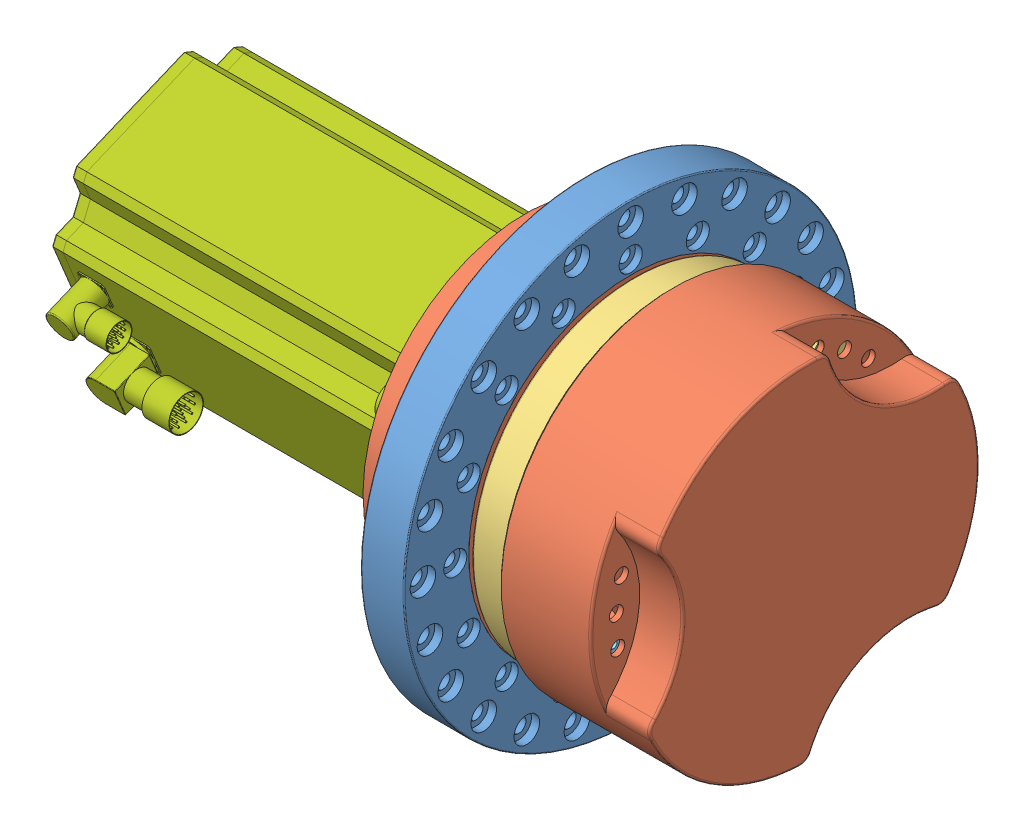
SolidWorks assembly GearBox2, configuration Default. Lengths in mm.
Overall size (603.55 457.3 457.3).
128 component instances, 22 part files, 59 mates.
Components (placement in the parent):
- Axis2_ConnectionRing1-1: Axis2_ConnectionRing1 [Default] at (258.0651 228.5311 262.5827) size (40 420 420)
- Axis2_GearBoxFixedPart-1: Axis2_GearBoxFixedPart [Default] at (233.3151 228.5311 262.5827) x (1 0 0) z (0 0.382683 -0.92388) size (225.2 350 350)
- RU_228X(GearBox2)-1: RU_228X(GearBox2) [Default] at (298.5651 228.5311 262.5827) x (-1 0 0) z (0 -0.957646 -0.287948) size (35 384.8 384.8) (flexible)
  - RU_228X_Outer(GearBox2)-1: RU_228X_Outer(GearBox2) [Default] x (1 0 0) z (0 0.3435 -0.939153) size (35 300 300)
  - RU_228X_Roller(GearBox2)-1: RU_228X_Roller(GearBox2) [Default] at (-8.75 -120.6811 -44.1397) size (9 9 9)
  - RU_228X_Inner(GearBox2)-1: RU_228X_Inner(GearBox2) [Default] x (1 0 0) z (0 -0.94978 -0.312918) size (35 254 254)
  - RU_228X_Roller(GearBox2)-3: RU_228X_Roller(GearBox2) [Default] at (8.75 -120.6811 -44.1397) x (-1 0 0) z (0 0 -1) size (9 9 9)
  - RU_228X_Roller(GearBox2)-4: RU_228X_Roller(GearBox2) [Default] at (8.75 -114.1974 -58.917) x (-1 0 0) z (0 0.125333 -0.992115) size (9 9 9)
  - RU_228X_Roller(GearBox2)-5: RU_228X_Roller(GearBox2) [Default] at (8.75 -105.9126 -72.7651) x (-1 0 0) z (0 0.24869 -0.968583) size (9 9 9)
  - RU_228X_Roller(GearBox2)-6: RU_228X_Roller(GearBox2) [Default] at (8.75 -95.9576 -85.4657) x (-1 0 0) z (0 0.368125 -0.929776) size (9 9 9)
  - RU_228X_Roller(GearBox2)-7: RU_228X_Roller(GearBox2) [Default] at (8.75 -84.4892 -96.8185) x (-1 0 0) z (0 0.481754 -0.876307) size (9 9 9)
  - RU_228X_Roller(GearBox2)-8: RU_228X_Roller(GearBox2) [Default] at (8.75 -71.6884 -106.6444) x (-1 0 0) z (0 0.587785 -0.809017) size (9 9 9)
  - RU_228X_Roller(GearBox2)-9: RU_228X_Roller(GearBox2) [Default] at (8.75 -57.7571 -114.7884) x (-1 0 0) z (0 0.684547 -0.728969) size (9 9 9)
  - RU_228X_Roller(GearBox2)-10: RU_228X_Roller(GearBox2) [Default] at (8.75 -42.9148 -121.1221) x (-1 0 0) z (0 0.770513 -0.637424) size (9 9 9)
  - RU_228X_Roller(GearBox2)-11: RU_228X_Roller(GearBox2) [Default] at (8.75 -27.3958 -125.5457) x (-1 0 0) z (0 0.844328 -0.535827) size (9 9 9)
  - RU_228X_Roller(GearBox2)-12: RU_228X_Roller(GearBox2) [Default] at (8.75 -11.4447 -127.9893) x (-1 0 0) z (0 0.904827 -0.425779) size (9 9 9)
  - RU_228X_Roller(GearBox2)-13: RU_228X_Roller(GearBox2) [Default] at (8.75 4.6868 -128.4145) x (-1 0 0) z (0 0.951057 -0.309017) size (9 9 9)
  - RU_228X_Roller(GearBox2)-14: RU_228X_Roller(GearBox2) [Default] at (8.75 20.7445 -126.8145) x (-1 0 0) z (0 0.982287 -0.187381) size (9 9 9)
  - RU_228X_Roller(GearBox2)-15: RU_228X_Roller(GearBox2) [Default] at (8.75 36.475 -123.2146) x (-1 0 0) z (0 0.998027 -0.062791) size (9 9 9)
  - RU_228X_Roller(GearBox2)-16: RU_228X_Roller(GearBox2) [Default] at (8.75 51.6302 -117.6714) x (-1 0 0) z (0 0.998027 0.062791) size (9 9 9)
  - RU_228X_Roller(GearBox2)-17: RU_228X_Roller(GearBox2) [Default] at (8.75 65.9712 -110.2726) x (-1 0 0) z (0 0.982287 0.187381) size (9 9 9)
  - RU_228X_Roller(GearBox2)-18: RU_228X_Roller(GearBox2) [Default] at (8.75 79.2719 -101.1347) x (-1 0 0) z (0 0.951057 0.309017) size (9 9 9)
  - RU_228X_Roller(GearBox2)-19: RU_228X_Roller(GearBox2) [Default] at (8.75 91.3223 -90.4018) x (-1 0 0) z (0 0.904827 0.425779) size (9 9 9)
  - RU_228X_Roller(GearBox2)-20: RU_228X_Roller(GearBox2) [Default] at (8.75 101.9326 -78.2432) x (-1 0 0) z (0 0.844328 0.535827) size (9 9 9)
  - RU_228X_Roller(GearBox2)-21: RU_228X_Roller(GearBox2) [Default] at (8.75 110.9353 -64.8507) x (-1 0 0) z (0 0.770513 0.637424) size (9 9 9)
  - RU_228X_Roller(GearBox2)-22: RU_228X_Roller(GearBox2) [Default] at (8.75 118.1885 -50.4355) x (-1 0 0) z (0 0.684547 0.728969) size (9 9 9)
  - RU_228X_Roller(GearBox2)-23: RU_228X_Roller(GearBox2) [Default] at (8.75 123.5778 -35.2248) x (-1 0 0) z (0 0.587785 0.809017) size (9 9 9)
  - RU_228X_Roller(GearBox2)-24: RU_228X_Roller(GearBox2) [Default] at (8.75 127.0181 -19.4587) x (-1 0 0) z (0 0.481754 0.876307) size (9 9 9)
  - RU_228X_Roller(GearBox2)-25: RU_228X_Roller(GearBox2) [Default] at (8.75 128.4554 -3.3856) x (-1 0 0) z (0 0.368125 0.929776) size (9 9 9)
  - RU_228X_Roller(GearBox2)-26: RU_228X_Roller(GearBox2) [Default] at (8.75 127.8668 12.7408) x (-1 0 0) z (0 0.24869 0.968583) size (9 9 9)
  - RU_228X_Roller(GearBox2)-27: RU_228X_Roller(GearBox2) [Default] at (8.75 125.2617 28.6663) x (-1 0 0) z (0 0.125333 0.992115) size (9 9 9)
  - RU_228X_Roller(GearBox2)-28: RU_228X_Roller(GearBox2) [Default] at (8.75 120.6811 44.1397) x (-1 0 0) z (0 0 1) size (9 9 9)
  - RU_228X_Roller(GearBox2)-29: RU_228X_Roller(GearBox2) [Default] at (8.75 114.1974 58.917) x (-1 0 0) z (0 -0.125333 0.992115) size (9 9 9)
  - RU_228X_Roller(GearBox2)-30: RU_228X_Roller(GearBox2) [Default] at (8.75 105.9126 72.7651) x (-1 0 0) z (0 -0.24869 0.968583) size (9 9 9)
  - RU_228X_Roller(GearBox2)-31: RU_228X_Roller(GearBox2) [Default] at (8.75 95.9576 85.4657) x (-1 0 0) z (0 -0.368125 0.929776) size (9 9 9)
  - RU_228X_Roller(GearBox2)-32: RU_228X_Roller(GearBox2) [Default] at (8.75 84.4892 96.8185) x (-1 0 0) z (0 -0.481754 0.876307) size (9 9 9)
  - RU_228X_Roller(GearBox2)-33: RU_228X_Roller(GearBox2) [Default] at (8.75 71.6884 106.6444) x (-1 0 0) z (0 -0.587785 0.809017) size (9 9 9)
  - RU_228X_Roller(GearBox2)-34: RU_228X_Roller(GearBox2) [Default] at (8.75 57.7571 114.7884) x (-1 0 0) z (0 -0.684547 0.728969) size (9 9 9)
  - RU_228X_Roller(GearBox2)-35: RU_228X_Roller(GearBox2) [Default] at (8.75 42.9148 121.1221) x (-1 0 0) z (0 -0.770513 0.637424) size (9 9 9)
  - RU_228X_Roller(GearBox2)-36: RU_228X_Roller(GearBox2) [Default] at (8.75 27.3958 125.5457) x (-1 0 0) z (0 -0.844328 0.535827) size (9 9 9)
  - RU_228X_Roller(GearBox2)-37: RU_228X_Roller(GearBox2) [Default] at (8.75 11.4447 127.9893) x (-1 0 0) z (0 -0.904827 0.425779) size (9 9 9)
  - RU_228X_Roller(GearBox2)-38: RU_228X_Roller(GearBox2) [Default] at (8.75 -4.6868 128.4145) x (-1 0 0) z (0 -0.951057 0.309017) size (9 9 9)
  - RU_228X_Roller(GearBox2)-39: RU_228X_Roller(GearBox2) [Default] at (8.75 -20.7445 126.8145) x (-1 0 0) z (0 -0.982287 0.187381) size (9 9 9)
  - RU_228X_Roller(GearBox2)-40: RU_228X_Roller(GearBox2) [Default] at (8.75 -36.475 123.2146) x (-1 0 0) z (0 -0.998027 0.062791) size (9 9 9)
  - RU_228X_Roller(GearBox2)-41: RU_228X_Roller(GearBox2) [Default] at (8.75 -51.6302 117.6714) x (-1 0 0) z (0 -0.998027 -0.062791) size (9 9 9)
  - RU_228X_Roller(GearBox2)-42: RU_228X_Roller(GearBox2) [Default] at (8.75 -65.9712 110.2726) x (-1 0 0) z (0 -0.982287 -0.187381) size (9 9 9)
  - RU_228X_Roller(GearBox2)-43: RU_228X_Roller(GearBox2) [Default] at (8.75 -79.2719 101.1347) x (-1 0 0) z (0 -0.951057 -0.309017) size (9 9 9)
  - RU_228X_Roller(GearBox2)-44: RU_228X_Roller(GearBox2) [Default] at (8.75 -91.3223 90.4018) x (-1 0 0) z (0 -0.904827 -0.425779) size (9 9 9)
  - RU_228X_Roller(GearBox2)-45: RU_228X_Roller(GearBox2) [Default] at (8.75 -101.9326 78.2432) x (-1 0 0) z (0 -0.844328 -0.535827) size (9 9 9)
  - RU_228X_Roller(GearBox2)-46: RU_228X_Roller(GearBox2) [Default] at (8.75 -110.9353 64.8507) x (-1 0 0) z (0 -0.770513 -0.637424) size (9 9 9)
  - RU_228X_Roller(GearBox2)-47: RU_228X_Roller(GearBox2) [Default] at (8.75 -118.1885 50.4355) x (-1 0 0) z (0 -0.684547 -0.728969) size (9 9 9)
  - RU_228X_Roller(GearBox2)-48: RU_228X_Roller(GearBox2) [Default] at (8.75 -123.5778 35.2248) x (-1 0 0) z (0 -0.587785 -0.809017) size (9 9 9)
  - RU_228X_Roller(GearBox2)-49: RU_228X_Roller(GearBox2) [Default] at (8.75 -127.0181 19.4587) x (-1 0 0) z (0 -0.481754 -0.876307) size (9 9 9)
  - RU_228X_Roller(GearBox2)-50: RU_228X_Roller(GearBox2) [Default] at (8.75 -128.4554 3.3856) x (-1 0 0) z (0 -0.368125 -0.929776) size (9 9 9)
  - RU_228X_Roller(GearBox2)-51: RU_228X_Roller(GearBox2) [Default] at (8.75 -127.8668 -12.7408) x (-1 0 0) z (0 -0.24869 -0.968583) size (9 9 9)
  - RU_228X_Roller(GearBox2)-52: RU_228X_Roller(GearBox2) [Default] at (8.75 -125.2617 -28.6663) x (-1 0 0) z (0 -0.125333 -0.992115) size (9 9 9)
  - RU_228X_Roller(GearBox2)-53: RU_228X_Roller(GearBox2) [Default] at (-8.75 -114.1974 -58.917) x (1 0 0) z (0 -0.125333 0.992115) size (9 9 9)
  - RU_228X_Roller(GearBox2)-54: RU_228X_Roller(GearBox2) [Default] at (-8.75 -105.9126 -72.7651) x (1 0 0) z (0 -0.24869 0.968583) size (9 9 9)
  - RU_228X_Roller(GearBox2)-55: RU_228X_Roller(GearBox2) [Default] at (-8.75 -95.9576 -85.4657) x (1 0 0) z (0 -0.368125 0.929776) size (9 9 9)
  - RU_228X_Roller(GearBox2)-56: RU_228X_Roller(GearBox2) [Default] at (-8.75 -84.4892 -96.8185) x (1 0 0) z (0 -0.481754 0.876307) size (9 9 9)
  - RU_228X_Roller(GearBox2)-57: RU_228X_Roller(GearBox2) [Default] at (-8.75 -71.6884 -106.6444) x (1 0 0) z (0 -0.587785 0.809017) size (9 9 9)
  - RU_228X_Roller(GearBox2)-58: RU_228X_Roller(GearBox2) [Default] at (-8.75 -57.7571 -114.7884) x (1 0 0) z (0 -0.684547 0.728969) size (9 9 9)
  - RU_228X_Roller(GearBox2)-59: RU_228X_Roller(GearBox2) [Default] at (-8.75 -42.9148 -121.1221) x (1 0 0) z (0 -0.770513 0.637424) size (9 9 9)
  - RU_228X_Roller(GearBox2)-60: RU_228X_Roller(GearBox2) [Default] at (-8.75 -27.3958 -125.5457) x (1 0 0) z (0 -0.844328 0.535827) size (9 9 9)
  - RU_228X_Roller(GearBox2)-61: RU_228X_Roller(GearBox2) [Default] at (-8.75 -11.4447 -127.9893) x (1 0 0) z (0 -0.904827 0.425779) size (9 9 9)
  - RU_228X_Roller(GearBox2)-62: RU_228X_Roller(GearBox2) [Default] at (-8.75 4.6868 -128.4145) x (1 0 0) z (0 -0.951057 0.309017) size (9 9 9)
  - RU_228X_Roller(GearBox2)-63: RU_228X_Roller(GearBox2) [Default] at (-8.75 20.7445 -126.8145) x (1 0 0) z (0 -0.982287 0.187381) size (9 9 9)
  - RU_228X_Roller(GearBox2)-64: RU_228X_Roller(GearBox2) [Default] at (-8.75 36.475 -123.2146) x (1 0 0) z (0 -0.998027 0.062791) size (9 9 9)
  - RU_228X_Roller(GearBox2)-65: RU_228X_Roller(GearBox2) [Default] at (-8.75 51.6302 -117.6714) x (1 0 0) z (0 -0.998027 -0.062791) size (9 9 9)
  - RU_228X_Roller(GearBox2)-66: RU_228X_Roller(GearBox2) [Default] at (-8.75 65.9712 -110.2726) x (1 0 0) z (0 -0.982287 -0.187381) size (9 9 9)
  - RU_228X_Roller(GearBox2)-67: RU_228X_Roller(GearBox2) [Default] at (-8.75 79.2719 -101.1347) x (1 0 0) z (0 -0.951057 -0.309017) size (9 9 9)
  - RU_228X_Roller(GearBox2)-68: RU_228X_Roller(GearBox2) [Default] at (-8.75 91.3223 -90.4018) x (1 0 0) z (0 -0.904827 -0.425779) size (9 9 9)
  - RU_228X_Roller(GearBox2)-69: RU_228X_Roller(GearBox2) [Default] at (-8.75 101.9326 -78.2432) x (1 0 0) z (0 -0.844328 -0.535827) size (9 9 9)
  - RU_228X_Roller(GearBox2)-70: RU_228X_Roller(GearBox2) [Default] at (-8.75 110.9353 -64.8507) x (1 0 0) z (0 -0.770513 -0.637424) size (9 9 9)
  - RU_228X_Roller(GearBox2)-71: RU_228X_Roller(GearBox2) [Default] at (-8.75 118.1885 -50.4355) x (1 0 0) z (0 -0.684547 -0.728969) size (9 9 9)
  - RU_228X_Roller(GearBox2)-72: RU_228X_Roller(GearBox2) [Default] at (-8.75 123.5778 -35.2248) x (1 0 0) z (0 -0.587785 -0.809017) size (9 9 9)
  - RU_228X_Roller(GearBox2)-73: RU_228X_Roller(GearBox2) [Default] at (-8.75 127.0181 -19.4587) x (1 0 0) z (0 -0.481754 -0.876307) size (9 9 9)
  - RU_228X_Roller(GearBox2)-74: RU_228X_Roller(GearBox2) [Default] at (-8.75 128.4554 -3.3856) x (1 0 0) z (0 -0.368125 -0.929776) size (9 9 9)
  - RU_228X_Roller(GearBox2)-75: RU_228X_Roller(GearBox2) [Default] at (-8.75 127.8668 12.7408) x (1 0 0) z (0 -0.24869 -0.968583) size (9 9 9)
  - RU_228X_Roller(GearBox2)-76: RU_228X_Roller(GearBox2) [Default] at (-8.75 125.2617 28.6663) x (1 0 0) z (0 -0.125333 -0.992115) size (9 9 9)
  - RU_228X_Roller(GearBox2)-77: RU_228X_Roller(GearBox2) [Default] at (-8.75 120.6811 44.1397) x (1 0 0) z (0 0 -1) size (9 9 9)
  - RU_228X_Roller(GearBox2)-78: RU_228X_Roller(GearBox2) [Default] at (-8.75 114.1974 58.917) x (1 0 0) z (0 0.125333 -0.992115) size (9 9 9)
  - RU_228X_Roller(GearBox2)-79: RU_228X_Roller(GearBox2) [Default] at (-8.75 105.9126 72.7651) x (1 0 0) z (0 0.24869 -0.968583) size (9 9 9)
  - RU_228X_Roller(GearBox2)-80: RU_228X_Roller(GearBox2) [Default] at (-8.75 95.9576 85.4657) x (1 0 0) z (0 0.368125 -0.929776) size (9 9 9)
  - RU_228X_Roller(GearBox2)-81: RU_228X_Roller(GearBox2) [Default] at (-8.75 84.4892 96.8185) x (1 0 0) z (0 0.481754 -0.876307) size (9 9 9)
  - RU_228X_Roller(GearBox2)-82: RU_228X_Roller(GearBox2) [Default] at (-8.75 71.6884 106.6444) x (1 0 0) z (0 0.587785 -0.809017) size (9 9 9)
  - RU_228X_Roller(GearBox2)-83: RU_228X_Roller(GearBox2) [Default] at (-8.75 57.7571 114.7884) x (1 0 0) z (0 0.684547 -0.728969) size (9 9 9)
  - RU_228X_Roller(GearBox2)-84: RU_228X_Roller(GearBox2) [Default] at (-8.75 42.9148 121.1221) x (1 0 0) z (0 0.770513 -0.637424) size (9 9 9)
  - RU_228X_Roller(GearBox2)-85: RU_228X_Roller(GearBox2) [Default] at (-8.75 27.3958 125.5457) x (1 0 0) z (0 0.844328 -0.535827) size (9 9 9)
  - RU_228X_Roller(GearBox2)-86: RU_228X_Roller(GearBox2) [Default] at (-8.75 11.4447 127.9893) x (1 0 0) z (0 0.904827 -0.425779) size (9 9 9)
  - RU_228X_Roller(GearBox2)-87: RU_228X_Roller(GearBox2) [Default] at (-8.75 -4.6868 128.4145) x (1 0 0) z (0 0.951057 -0.309017) size (9 9 9)
  - RU_228X_Roller(GearBox2)-88: RU_228X_Roller(GearBox2) [Default] at (-8.75 -20.7445 126.8145) x (1 0 0) z (0 0.982287 -0.187381) size (9 9 9)
  - RU_228X_Roller(GearBox2)-89: RU_228X_Roller(GearBox2) [Default] at (-8.75 -36.475 123.2146) x (1 0 0) z (0 0.998027 -0.062791) size (9 9 9)
  - RU_228X_Roller(GearBox2)-90: RU_228X_Roller(GearBox2) [Default] at (-8.75 -51.6302 117.6714) x (1 0 0) z (0 0.998027 0.062791) size (9 9 9)
  - RU_228X_Roller(GearBox2)-91: RU_228X_Roller(GearBox2) [Default] at (-8.75 -65.9712 110.2726) x (1 0 0) z (0 0.982287 0.187381) size (9 9 9)
  - RU_228X_Roller(GearBox2)-92: RU_228X_Roller(GearBox2) [Default] at (-8.75 -79.2719 101.1347) x (1 0 0) z (0 0.951057 0.309017) size (9 9 9)
  - RU_228X_Roller(GearBox2)-93: RU_228X_Roller(GearBox2) [Default] at (-8.75 -91.3223 90.4018) x (1 0 0) z (0 0.904827 0.425779) size (9 9 9)
  - RU_228X_Roller(GearBox2)-94: RU_228X_Roller(GearBox2) [Default] at (-8.75 -101.9326 78.2432) x (1 0 0) z (0 0.844328 0.535827) size (9 9 9)
  - RU_228X_Roller(GearBox2)-95: RU_228X_Roller(GearBox2) [Default] at (-8.75 -110.9353 64.8507) x (1 0 0) z (0 0.770513 0.637424) size (9 9 9)
  - RU_228X_Roller(GearBox2)-96: RU_228X_Roller(GearBox2) [Default] at (-8.75 -118.1885 50.4355) x (1 0 0) z (0 0.684547 0.728969) size (9 9 9)
  - RU_228X_Roller(GearBox2)-97: RU_228X_Roller(GearBox2) [Default] at (-8.75 -123.5778 35.2248) x (1 0 0) z (0 0.587785 0.809017) size (9 9 9)
  - RU_228X_Roller(GearBox2)-98: RU_228X_Roller(GearBox2) [Default] at (-8.75 -127.0181 19.4587) x (1 0 0) z (0 0.481754 0.876307) size (9 9 9)
  - RU_228X_Roller(GearBox2)-99: RU_228X_Roller(GearBox2) [Default] at (-8.75 -128.4554 3.3856) x (1 0 0) z (0 0.368125 0.929776) size (9 9 9)
  - RU_228X_Roller(GearBox2)-100: RU_228X_Roller(GearBox2) [Default] at (-8.75 -127.8668 -12.7408) x (1 0 0) z (0 0.24869 0.968583) size (9 9 9)
  - RU_228X_Roller(GearBox2)-101: RU_228X_Roller(GearBox2) [Default] at (-8.75 -125.2617 -28.6663) x (1 0 0) z (0 0.125333 0.992115) size (9 9 9)
- KSSG1.5-22-J30-1: KSSG1.5-22-J30 [Default] at (278.0651 228.5311 262.5827) x (0 0.892284 -0.451475) z (0 0.451475 0.892284) size (62.94 55.14 62.99)
- Servo_Axis_1-2-3-1: Servo_Axis_1-2-3 [Default] at (-149.4349 228.5311 262.5827) x (0 -0.92388 -0.382683) z (0 -0.382683 0.92388) size (190 412 229) (flexible)
  - AEG-69-225-468_6,6kW_21-Nm-1: AEG-69-225-468_6,6kW_21-Nm [Default] at origin size (190 342 229)
  - ServoShaft_30mm-1: ServoShaft_30mm [Default] at (0 69 0) x (-0.651591 0 -0.75857) z (0.75857 0 -0.651591) size (30 330 30)
  - SKF_16006-1: SKF_16006 [Default] at (0 320.5 0) x (0 1 0) z (-0.999913 0 0.013216) size (9 55 55)
- KSSAY0.8-20-K10-1: KSSAY0.8-20-K10 [Default] at (267.5651 247.2826 217.3126) x (0 0.964181 -0.265245) z (0 0.265245 0.964181) size (39.87 130 39.97)
- SKF_61807-2: SKF_61807 [Default] at (239.5651 228.5311 262.5827) x (1 0 0) z (0 0.25232 -0.967644) size (7.4 48.24 48.12)
- SKF_61804-2: SKF_61804 [Default] at (236.0651 247.2826 217.3126) size (7.11 32.85 32.78)
- SKF_61807-3: SKF_61807 [Default] at (232.5651 228.5311 262.5827) size (7.4 48.24 48.12)
- SKF_61804-3: SKF_61804 [Default] at (316.5651 247.2826 217.3126) x (1 0 0) z (0 0.018942 -0.999821) size (7.11 32.85 32.78)
- SKF_16006-1: SKF_16006 [Default] at (184.0651 228.5311 262.5827) x (1 0 0) z (0 0.036218 0.999344) size (9 55 55)
- mmsa2-20R_BevelGear(GearBox2)-1: mmsa2-20R_BevelGear(GearBox2) [Default] at (344.5651 247.2826 217.3126) x (0 0.964181 -0.265245) z (0 -0.265245 -0.964181) size (54.75 25.25 51.87)
- mmsa2-20L_BevelGear(GearBox2)-1: mmsa2-20L_BevelGear(GearBox2) [Default] at (380.2651 261.0592 184.053) x (-0.557221 -0.767156 -0.317767) z (-0.830364 0.514805 0.213239) size (54.26 25.25 51.03)
- GearBox2_BevelShaft-1: GearBox2_BevelShaft [Default] at (380.2651 189.4974 356.8184) x (0.557221 0.767156 0.317767) z (-0.830364 0.514805 0.213239) size (15 204 15)
- SKF_61902-1: SKF_61902 [Default] at (380.2651 193.8982 346.1938) x (0 -0.382683 0.92388) z (-0.92388 0.353553 0.146447) size (7.1 28.75 28.69)
- SKF_61902-2: SKF_61902 [Default] at (380.2651 263.1639 178.9716) x (0 -0.382683 0.92388) z (-0.92388 0.353553 0.146447) size (7.1 28.75 28.69)
- AGDL2-50R1_WormWheel(GearBox2)-1: AGDL2-50R1_WormWheel(GearBox2) [Default] at (387.7651 147.497 283.1369) x (1 0 0) z (0 -0.594678 -0.803964) size (37.78 108.94 108.94)
- KWGDL2-R1_WormGear(Gearbox2)-1: KWGDL2-R1_WormGear(Gearbox2) [Default] at (380.2651 229.2964 260.735) x (0.557221 0.767156 0.317767) z (0.830364 -0.514805 -0.213239) size (38.22 84 44.07)
- WormWheelShaft(GearBox2)-1: WormWheelShaft(GearBox2) [Default] at (423.9151 147.497 283.1369) x (0 0.594678 0.803964) z (0 -0.803964 0.594678) size (30 109.85 30)
- SKF_61902-3: SKF_61902 [Default] at (317.5651 147.497 283.1369) x (-1 0 0) z (0 0.999977 -0.006841) size (7.1 28.75 28.69)
- GearBox_2_Top-1: GearBox_2_Top [Default] at (441.0651 228.5311 262.5827) x (0 -0.998286 0.058524) z (0 -0.058524 -0.998286) size (321.81 125.05 320)
- SSR2.5-90_InternalSpurGear(GearBox2)-1: SSR2.5-90_InternalSpurGear(GearBox2) [Default] at (338.5651 228.5311 262.5827) x (0 -0.664512 0.747277) z (-1 0 0) size (300 300 25)
- SSA2-55(GearBox2)-1: SSA2-55(GearBox2) [Default] at (346.9151 147.497 283.1369) x (0 0.594678 0.803964) z (0 -0.803964 0.594678) size (84 20.1 83.74)
Mates (geometry in assembly coordinates):
- Concentric1: concentric aligned: cylinder of Axis2_ConnectionRing1-1 through (258.0651 228.5311 262.5827) axis (1 0 0) radius 175; cylinder of Axis2_GearBoxFixedPart-1 through (278.0651 228.5311 262.5827) axis (1 0 0) radius 150
- Coincident1: coincident anti-aligned: plane of Axis2_ConnectionRing1-1 through (263.0651 378.5311 262.5827) normal (-1 0 0); plane of Axis2_GearBoxFixedPart-1 through (263.0651 228.5311 262.5827) normal (1 0 0)
- Concentric6: concentric aligned: cylinder of Axis2_GearBoxFixedPart-1 through (263.0651 78.4006 324.7688) axis (1 0 0) radius 6; cylinder of Axis2_ConnectionRing1-1 through (278.0651 78.4006 324.7688) axis (1 0 0) radius 6
- Concentric7: concentric anti-aligned: cylinder of Axis2_ConnectionRing1-1 through (258.0651 228.5311 262.5827) axis (1 0 0) radius 210; cylinder of RU_228X(GearBox2)-1/RU_228X_Inner(GearBox2)-1 through (298.5651 228.5311 262.5827) axis (-1 0 0) radius 105
- Coincident4: coincident anti-aligned: plane of Axis2_GearBoxFixedPart-1 through (281.0651 228.5311 262.5827) normal (1 0 0); plane of RU_228X(GearBox2)-1/RU_228X_Inner(GearBox2)-1 through (281.0651 228.5311 262.5827) normal (-1 0 0)
- Concentric12: concentric aligned: cylinder of Axis2_GearBoxFixedPart-1 through (281.0651 112.5708 265.6192) axis (1 0 0) radius 3.3; cylinder of RU_228X(GearBox2)-1/RU_228X_Inner(GearBox2)-1 through (316.0651 112.5708 265.6192) axis (1 0 0) radius 3.3
- Concentric17: concentric anti-aligned: cylinder of KSSG1.5-22-J30-1 through (250.0651 228.5311 262.5827) axis (-1 0 0) radius 17.5; cylinder of SKF_61807-2 through (239.5651 228.5311 262.5827) axis (1 0 0) radius 17.5
- Coincident9: coincident anti-aligned: plane of KSSG1.5-22-J30-1 through (243.0651 220.6303 246.9678) normal (-1 0 0); plane of SKF_61807-2 through (243.0651 228.5311 262.5827) normal (1 0 0)
- Concentric18: concentric anti-aligned: cylinder of KSSG1.5-22-J30-1 through (250.0651 228.5311 262.5827) axis (-1 0 0) radius 17.5; cylinder of SKF_61807-3 through (232.5651 228.5311 262.5827) axis (1 0 0) radius 17.5
- Coincident10: coincident anti-aligned: plane of SKF_61807-2 through (236.0651 228.5311 262.5827) normal (-1 0 0); plane of SKF_61807-3 through (236.0651 228.5311 262.5827) normal (1 0 0)
- Concentric19: concentric anti-aligned: cylinder of KSSAY0.8-20-K10-1 through (362.5651 247.2826 217.3126) axis (-1 0 0) radius 10; cylinder of SKF_61804-2 through (236.0651 247.2826 217.3126) axis (1 0 0) radius 10
- Coincident11: coincident aligned: plane of KSSAY0.8-20-K10-1 through (232.5651 247.2826 217.3126) normal (-1 0 0); plane of SKF_61804-2 through (232.5651 247.2826 217.3126) normal (-1 0 0)
- Concentric20: concentric anti-aligned: cylinder of KSSAY0.8-20-K10-1 through (362.5651 247.2826 217.3126) axis (-1 0 0) radius 10; cylinder of SKF_61804-3 through (316.5651 247.2826 217.3126) axis (1 0 0) radius 10
- Concentric21: concentric aligned: cylinder of Axis2_GearBoxFixedPart-1 through (321.0651 247.2826 217.3126) axis (1 0 0) radius 11; cylinder of SKF_61804-2 through (236.0651 247.2826 217.3126) axis (1 0 0) radius 16
- Coincident14: coincident anti-aligned: plane of Axis2_GearBoxFixedPart-1 through (232.5651 247.2826 217.3126) normal (1 0 0); plane of SKF_61804-2 through (232.5651 247.2826 217.3126) normal (-1 0 0)
- Coincident15: coincident anti-aligned: plane of Axis2_GearBoxFixedPart-1 through (313.0651 237.1199 213.1031) normal (1 0 0); plane of SKF_61804-3 through (313.0651 247.2826 217.3126) normal (-1 0 0)
- Concentric22: concentric anti-aligned: cylinder of Axis2_GearBoxFixedPart-1 through (180.0651 228.5311 262.5827) axis (-1 0 0) radius 23.5; cylinder of SKF_61807-2 through (239.5651 228.5311 262.5827) axis (1 0 0) radius 23.5
- Coincident16: coincident anti-aligned: plane of Axis2_GearBoxFixedPart-1 through (229.0651 212.3632 255.8858) normal (1 0 0); plane of SKF_61807-3 through (229.0651 228.5311 262.5827) normal (-1 0 0)
- Concentric23: concentric anti-aligned: cylinder of Axis2_GearBoxFixedPart-1 through (278.0651 228.5311 262.5827) axis (1 0 0) radius 27.5; cylinder of SKF_16006-1 through (184.0651 228.5311 262.5827) axis (-1 0 0) radius 27.5
- Coincident17: coincident anti-aligned: plane of Axis2_GearBoxFixedPart-1 through (188.5651 228.5311 262.5827) normal (-1 0 0); plane of SKF_16006-1 through (188.5651 228.5311 262.5827) normal (1 0 0)
- Concentric24: concentric aligned: cylinder of Servo_Axis_1-2-3-1/ServoShaft_30mm-1 through (-80.4349 228.5311 262.5827) axis (-1 0 0) radius 15; cylinder of SKF_16006-1 through (184.0651 228.5311 262.5827) axis (-1 0 0) radius 15
- Coincident18: coincident anti-aligned: plane of KSSG1.5-22-J30-1 through (278.0651 228.5311 262.5827) normal (0 0.451475 0.892284); plane of Servo_Axis_1-2-3-1/ServoShaft_30mm-1 through (-80.4349 228.5311 262.5827) normal (0 -0.451475 -0.892284)
- Coincident19: coincident anti-aligned: plane of Axis2_GearBoxFixedPart-1 through (179.5651 228.5311 262.5827) normal (-1 0 0); plane of Servo_Axis_1-2-3-1/AEG-69-225-468_6,6kW_21-Nm-1 through (179.5651 228.5311 262.5827) normal (1 0 0)
- Concentric25: concentric anti-aligned: cylinder of Axis2_GearBoxFixedPart-1 through (200.5651 269.0955 360.514) axis (-1 0 0) radius 8.5; cylinder of Servo_Axis_1-2-3-1/AEG-69-225-468_6,6kW_21-Nm-1 through (-149.4359 269.0955 360.514) axis (1 0 0) radius 8.5
- GearMate1: gear = 35 : 21 mm: cylinder of KSSAY0.8-20-K10-1 through (262.5651 247.2826 217.3126) axis (1 0 0) radius 20; cylinder of KSSG1.5-22-J30-1 through (258.0651 228.5311 262.5827) axis (1 0 0) radius 31.5
- Coincident20: coincident anti-aligned: plane of KSSAY0.8-20-K10-1 through (344.5651 247.3459 217.2952) normal (1 0 0); plane of mmsa2-20R_BevelGear(GearBox2)-1 through (344.5651 247.2826 217.3126) normal (-1 0 0)
- Concentric26: concentric anti-aligned: cylinder of KSSAY0.8-20-K10-1 through (344.5651 247.2826 217.3126) axis (1 0 0) radius 7.5; cylinder of mmsa2-20R_BevelGear(GearBox2)-1 through (344.5651 247.2826 217.3126) axis (-1 0 0) radius 7.5
- Coincident21: coincident aligned: plane of KSSAY0.8-20-K10-1 through (340.3225 251.116 225.5924) normal (0 -0.964181 0.265245); plane of mmsa2-20R_BevelGear(GearBox2)-1 through (344.5651 251.116 225.5924) normal (0 -0.964181 0.265245)
- Concentric28: concentric anti-aligned: cylinder of Axis2_GearBoxFixedPart-1 through (380.2651 267.5648 168.347) axis (0 -0.382683 0.92388) radius 8.5; cylinder of mmsa2-20L_BevelGear(GearBox2)-1 through (380.2651 261.0592 184.053) axis (0 0.382683 -0.92388) radius 7.5
- Concentric29: concentric anti-aligned: cylinder of Axis2_GearBoxFixedPart-1 through (380.2651 267.5648 168.347) axis (0 -0.382683 0.92388) radius 8.5; cylinder of GearBox2_BevelShaft-1 through (380.2651 267.5648 168.347) axis (0 0.382683 -0.92388) radius 7.5
- Coincident22: coincident aligned: plane of Axis2_GearBoxFixedPart-1 through (380.2651 267.5648 168.347) normal (0 0.382683 -0.92388); plane of GearBox2_BevelShaft-1 through (384.4443 273.3184 170.7303) normal (0 0.382683 -0.92388)
- Coincident25: coincident aligned: plane of mmsa2-20L_BevelGear(GearBox2)-1 through (388.5742 257.5766 182.6105) normal (-0.557221 -0.767156 -0.317767); plane of GearBox2_BevelShaft-1 through (388.5742 250.6883 199.2403) normal (-0.557221 -0.767156 -0.317767)
- Coincident26: coincident anti-aligned: plane of mmsa2-20L_BevelGear(GearBox2)-1 through (380.2651 261.0592 184.053) normal (0 0.382683 -0.92388); plane of GearBox2_BevelShaft-1 through (380.2651 261.0592 184.053) normal (0 -0.382683 0.92388)
- GearMate2: gear = 35 : 35 mm: circle of mmsa2-20L_BevelGear(GearBox2)-1; circle of mmsa2-20R_BevelGear(GearBox2)-1
- Concentric30: concentric anti-aligned: cylinder of GearBox2_BevelShaft-1 through (380.2651 267.5648 168.347) axis (0 0.382683 -0.92388) radius 7.5; cylinder of SKF_61902-1 through (380.2651 193.8982 346.1938) axis (0 -0.382683 0.92388) radius 7.5
- Coincident27: coincident anti-aligned: plane of Axis2_GearBoxFixedPart-1 through (380.2651 192.5588 349.4274) normal (0 0.382683 -0.92388); plane of SKF_61902-1 through (380.2651 192.5588 349.4274) normal (0 -0.382683 0.92388)
- Concentric31: concentric anti-aligned: cylinder of GearBox2_BevelShaft-1 through (380.2651 267.5648 168.347) axis (0 0.382683 -0.92388) radius 7.5; cylinder of SKF_61902-2 through (380.2651 263.1639 178.9716) axis (0 -0.382683 0.92388) radius 7.5
- Coincident28: coincident anti-aligned: plane of Axis2_GearBoxFixedPart-1 through (380.2651 264.5033 175.738) normal (0 -0.382683 0.92388); plane of SKF_61902-2 through (380.2651 264.5033 175.738) normal (0 0.382683 -0.92388)
- Concentric32: concentric anti-aligned: cylinder of Axis2_GearBoxFixedPart-1 through (314.0651 147.497 283.1369) axis (1 0 0) radius 14; cylinder of SKF_61902-3 through (317.5651 147.497 283.1369) axis (-1 0 0) radius 7.5
- Coincident29: coincident anti-aligned: plane of Axis2_GearBoxFixedPart-1 through (314.0651 147.497 283.1369) normal (1 0 0); plane of SKF_61902-3 through (314.0651 147.497 283.1369) normal (-1 0 0)
- Concentric33: concentric aligned: cylinder of WormWheelShaft(GearBox2)-1 through (314.0651 147.497 283.1369) axis (-1 0 0) radius 7.5; cylinder of SKF_61902-3 through (317.5651 147.497 283.1369) axis (-1 0 0) radius 7.5
- Coincident31: coincident aligned: plane of AGDL2-50R1_WormWheel(GearBox2)-1 through (368.8303 139.1172 291.3565) normal (0 -0.594678 -0.803964); plane of WormWheelShaft(GearBox2)-1 through (364.3189 139.1172 291.3565) normal (0 -0.594678 -0.803964)
- Coincident32: coincident anti-aligned: plane of AGDL2-50R1_WormWheel(GearBox2)-1 through (368.9151 139.4573 289.0837) normal (-1 0 0); plane of WormWheelShaft(GearBox2)-1 through (368.9151 153.4437 291.1765) normal (1 0 0)
- Concentric34: concentric aligned: cylinder of AGDL2-50R1_WormWheel(GearBox2)-1 through (387.7651 147.497 283.1369) axis (-1 0 0) radius 10; cylinder of WormWheelShaft(GearBox2)-1 through (314.0651 147.497 283.1369) axis (-1 0 0) radius 7.5
- Concentric35: concentric aligned: cylinder of GearBox2_BevelShaft-1 through (380.2651 267.5648 168.347) axis (0 0.382683 -0.92388) radius 7.5; cylinder of KWGDL2-R1_WormGear(Gearbox2)-1 through (380.2651 229.2964 260.735) axis (0 0.382683 -0.92388) radius 15
- Coincident33: coincident aligned: plane of GearBox2_BevelShaft-1 through (388.5742 220.0737 273.1507) normal (-0.557221 -0.767156 -0.317767); plane of KWGDL2-R1_WormGear(Gearbox2)-1 through (388.5742 218.4501 277.0703) normal (-0.557221 -0.767156 -0.317767)
- Coincident34: coincident anti-aligned: plane of GearBox2_BevelShaft-1 through (380.2651 229.2964 260.735) normal (0 -0.382683 0.92388); plane of KWGDL2-R1_WormGear(Gearbox2)-1 through (380.2651 229.2964 260.735) normal (0 0.382683 -0.92388)
- Coincident35: coincident: plane of AGDL2-50R1_WormWheel(GearBox2)-1 through (380.2651 147.497 283.1369) normal (1 0 0); line of KWGDL2-R1_WormGear(Gearbox2)-1 through (380.2651 197.151 338.3408) axis (0 0.382683 -0.92388)
- GearMate3: gear = 25 : 40 mm: cylinder of AGDL2-50R1_WormWheel(GearBox2)-1 through (387.7651 147.497 283.1369) axis (-1 0 0) radius 20; cylinder of KWGDL2-R1_WormGear(Gearbox2)-1 through (380.2651 229.2964 260.735) axis (0 0.382683 -0.92388) radius 12.5
- Coincident39: coincident anti-aligned: line of RU_228X(GearBox2)-1 through (317.8151 228.5311 262.5827) axis (-1 0 0); line of SSR2.5-90_InternalSpurGear(GearBox2)-1 through (326.0651 228.5311 262.5827) axis (1 0 0)
- Concentric37: concentric aligned: cylinder of RU_228X(GearBox2)-1/RU_228X_Outer(GearBox2)-1 through (281.0651 333.1499 355.6144) axis (-1 0 0) radius 3.3; cylinder of SSR2.5-90_InternalSpurGear(GearBox2)-1 through (351.0651 333.1499 355.6144) axis (-1 0 0) radius 3.3
- Coincident40: coincident aligned: line of GearBox_2_Top-1 through (316.0651 228.5311 262.5827) axis (1 0 0); line of SSR2.5-90_InternalSpurGear(GearBox2)-1 through (326.0651 228.5311 262.5827) axis (1 0 0)
- Coincident41: coincident anti-aligned: plane of GearBox_2_Top-1 through (326.0651 228.5311 262.5827) normal (1 0 0); plane of SSR2.5-90_InternalSpurGear(GearBox2)-1 through (326.0651 228.5311 262.5827) normal (-1 0 0)
- Concentric38: concentric aligned: cylinder of GearBox_2_Top-1 through (441.0661 236.7244 402.3428) axis (-1 0 0) radius 3.3; cylinder of SSR2.5-90_InternalSpurGear(GearBox2)-1 through (351.0651 236.7244 402.3428) axis (-1 0 0) radius 3.3
- Coincident42: coincident anti-aligned: plane of RU_228X(GearBox2)-1/RU_228X_Outer(GearBox2)-1 through (316.0651 228.5311 262.5827) normal (1 0 0); plane of GearBox_2_Top-1 through (316.0651 228.5311 262.5827) normal (-1 0 0)
- Concentric40: concentric aligned: cylinder of WormWheelShaft(GearBox2)-1 through (314.0651 147.497 283.1369) axis (-1 0 0) radius 10; cylinder of SSA2-55(GearBox2)-1 through (356.9651 147.497 283.1369) axis (-1 0 0) radius 9
- Coincident45: coincident aligned: plane of WormWheelShaft(GearBox2)-1 through (361.5113 155.0727 275.512) normal (0 0.594678 0.803964); plane of SSA2-55(GearBox2)-1 through (356.9651 146.5306 281.8305) normal (0 0.594678 0.803964)
- Coincident47: coincident anti-aligned: plane of WormWheelShaft(GearBox2)-1 through (356.9151 156.4171 295.1964) normal (-1 0 0); plane of SSA2-55(GearBox2)-1 through (356.9151 147.497 283.1369) normal (1 0 0)
- GearMate4: gear = 90 : 30 mm: circle of SSA2-55(GearBox2)-1; circle of SSR2.5-90_InternalSpurGear(GearBox2)-1
